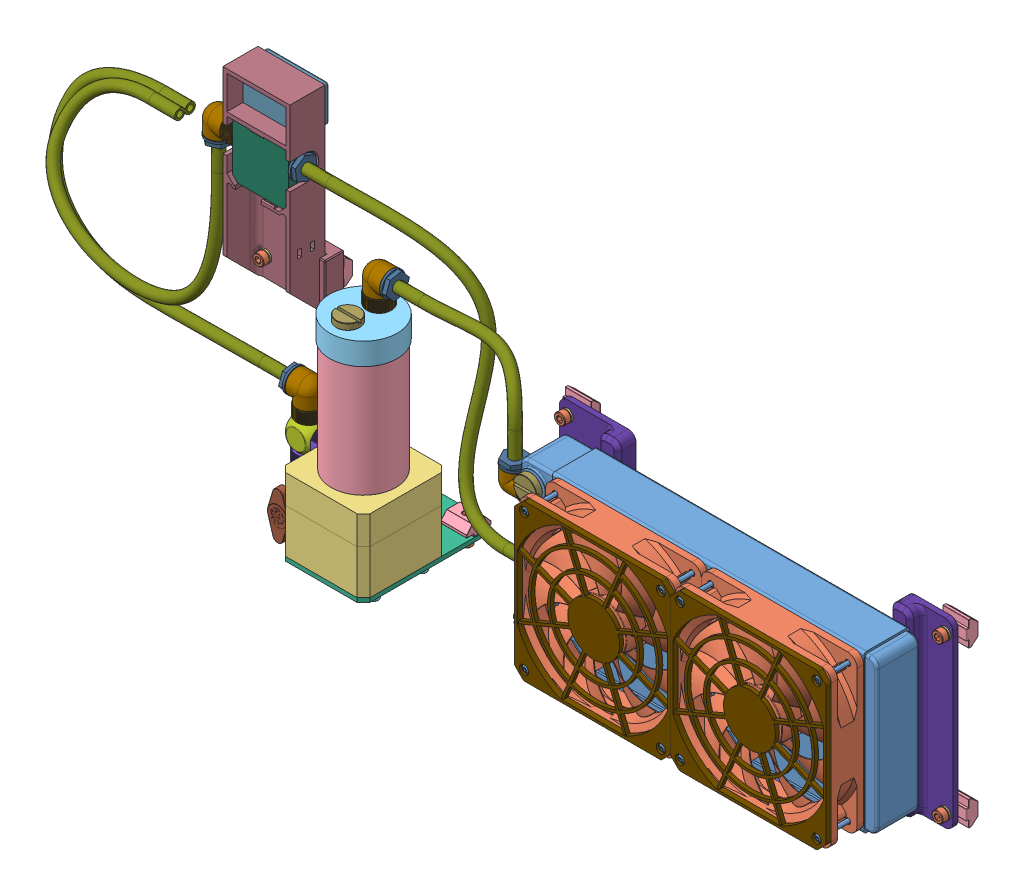
SolidWorks assembly Spindle Cooling Radiator System, configuration Default. Lengths in mm.
Overall size (706.65 292.49 113).
80 component instances, 24 part files, 129 mates.
Components (placement in the parent):
- XSPC EX240 Radiator-1: XSPC EX240 Radiator [Default] at (629 19.5 31.5) x (0 1 0) z (0 0 1) size (121 276 36)
- Noctua_nf-p12 redux-1700-1: Noctua_nf-p12 redux-1700 [Default] at (559.8 79.8 74) x (-1 0 0) z (0 0 -1) size (120 120.2 29.18)
- Noctua_nf-p12 redux-1700-2: Noctua_nf-p12 redux-1700 [Default] at (439.8 79.8 74) x (-1 0 0) z (0 0 -1) size (120 120.2 29.18)
- Cooling Pump-1: Cooling Pump [Default] at (220 0 34.5) x (0 0 1) z (-1 0 0) size (102 211.26 121.52)
  - Freezemod_PU-FS6M-1: Freezemod_PU-FS6M [Default] at origin size (65 159.5 65)
    - Freezemod FS6M_Plus-1: Freezemod FS6M_Plus [Default] at origin size (65 56 65)
    - Freezemod Resevoir-1: Freezemod Resevoir [Default] at (0 99.5 0) x (1 0 0) z (0 1 0) size (52 52 110.5)
      - Innter Tube-1: Innter Tube [Default] at (0 0 99.5) x (1 0 0) z (0 0 -1) size (50 50 100)
      - Top Cap-1: Top Cap [Default] at (0 0 60) x (1 0 0) z (0 0 -1) size (52 52 17)
  - Freezemod PU-FS6M Mounting Bracket-1: Freezemod PU-FS6M Mounting Bracket [Default] at (-18.5 0 0) x (0 0 1) z (0 -1 0) size (65 102 3.17)
  - Bitspower_T_Fitting-1: Bitspower_T_Fitting [Défaut] at (-16.5 43 58.66) x (0 0 1) z (1 0 0) size (25.4 20.32 25.4)
  - EK-AF Extender Rotary M-M G1_4-1: EK-AF Extender Rotary M-M G1_4 [Default] at (-16.5 43 48.5) x (1 0 0) z (0 1 0) size (19.99 25.44 20)
  - EK-AF Angled 90deg G1_4-1: EK-AF Angled 90deg G1_4 [Default] at (-16.5 53.66 58.66) x (-1 0 0) z (0 0 -1) size (19 36.31 19.39)
  - G14x6mm_Barb-1: G14x6mm_Barb [Défaut] at (-16.5 72.46 73.0225) x (0 0 1) z (-0.923728 -0.383049 0) size (25.52 18.33 18.33)
  - EK-AF Extender Rotary M-M G1_4-2: EK-AF Extender Rotary M-M G1_4 [Default] at (-16.5 16.84 58.66) size (19.99 25.44 20)
  - G14_Valve-1: G14_Valve [Predeterminado] at (-16.5 -1.16 58.66) x (0 0 -1) z (0 -1 0) size (23 35.7 37.13)
  - G14_Plug-1: G14_Plug [Default] at (12 165.3 0) x (1 0 0) z (0 -1 0) size (18.01 18.01 9.94)
  - EK-AF Angled 90deg G1_4-3: EK-AF Angled 90deg G1_4 [Default] at (-12 160 0) size (19 36.31 19.39)
  - G14x6mm_Barb-2: G14x6mm_Barb [Défaut] at (-12 178.8 -14.3625) x (0 0 -1) z (-0.216826 -0.97621 0) size (25.52 18.33 18.33)
- G14x6mm_Barb-1: G14x6mm_Barb [Défaut] at (348.2375 55 31.5) x (-1 0 0) z (0 -0.924225 -0.381849) size (25.52 18.33 18.33)
- Flow_Temp_Indicator_ASMB-1: Flow_Temp_Indicator_ASMB [Default] at (140 256.91 10) x (-1 0 0) z (0 0 -1) size (96.24 147.76 37.92)
  - Flow Meter And Temp Gauge-1: Flow Meter And Temp Gauge [Default] at origin size (61.6 147.76 37)
  - Fosa Pointer Display Thermometer-1: Fosa Pointer Display Thermometer [Défaut] at origin size (48 28 20)
  - Fosa G14 Flow Meter-1: Fosa G14 Flow Meter [Default] at (0 -37.73 -4) size (43.25 43.13 20)
  - EK-AF Angled 90deg G1_4-1: EK-AF Angled 90deg G1_4 [Default] at (22.125 -32.1 -15) x (0 0 1) z (0 1 0) size (19 36.31 19.39)
  - G14x6mm_Barb-1: G14x6mm_Barb [Défaut] at (-26.3875 -32.1 -15) x (-1 0 0) z (0 -0.924225 -0.381849) size (25.52 18.33 18.33)
  - G14x6mm_Barb-2: G14x6mm_Barb [Défaut] at (40.925 -46.4625 -15) x (0 -1 0) z (-0.650255 0 0.759716) size (25.52 18.33 18.33)
- EK-AF Angled 90deg G1_4-1: EK-AF Angled 90deg G1_4 [Default] at (352.5 105 31.5) x (0 0 1) z (0 -1 0) size (19 36.31 19.39)
- G14x6mm_Barb-2: G14x6mm_Barb [Défaut] at (333.7 119.3625 31.5) x (0 1 0) z (0 0 1) size (25.52 18.33 18.33)
- Water Cooling Tubes-1: Water Cooling Tubes [Default] at (333.7 119.3625 31.5) x (0 0 -1) z (0 1 0) size (64.89 407.39 178.39)
- G14_Plug-1: G14_Plug [Default] at (365 125 55.3) x (0 1 0) z (0 0 -1) size (18.01 18.01 9.94)
- G14_Plug-2: G14_Plug [Default] at (365 35 55.3) x (-0.158553 0.987351 0) z (0 0 -1) size (18.01 18.01 9.94)
- Radiator Mount-1: Radiator Mount [Outlet Side] at (368 80 0) x (0 1 0) z (0 0 1) size (140 55 14)
- Radiator Mount-2: Radiator Mount [Default] at (624 80 0) x (0 -1 0) z (0 0 1) size (140 39 14)
- Fan_Grill-1: Fan_Grill [Default] at (439.8 79.8 74) size (120 120 4)
- Fan_Grill-2: Fan_Grill [Default] at (559.8 79.8 74) size (120 120 4)
- Trimcraft M3 BSC-1: Trimcraft M3 BSC [3mm x 06mm SST BSC] at (387.5 132.5 9.35) x (-0.923728 -0.383049 0) z (0 0 -1) size (5.7 5.7 7.77)
- Trimcraft M3 BSC-2: Trimcraft M3 BSC [3mm x 06mm SST BSC] at (387.5 27.5 9.35) x (-0.85131 -0.524663 0) z (0 0 -1) size (5.7 5.7 7.77)
- Trimcraft M3 BSC-5: Trimcraft M3 BSC [3mm x 06mm SST BSC] at (612.5 132.5 9.35) x (-0.777574 -0.628792 0) z (0 0 -1) size (5.7 5.7 7.77)
- Trimcraft M3 BSC-7: Trimcraft M3 BSC [3mm x 06mm SST BSC] at (612.5 27.5 9.35) x (-0.715577 -0.698533 0) z (0 0 -1) size (5.7 5.7 7.77)
- Trimcraft M3 BSC-10: Trimcraft M3 BSC [3mm x 30mm SST BSC] at (387.1 27.1 77.65) size (5.7 5.7 31.77)
- Trimcraft M3 BSC-11: Trimcraft M3 BSC [3mm x 30mm SST BSC] at (387.1 132.5 77.65) x (0.987351 0.158553 0) z (0 0 1) size (5.7 5.7 31.77)
- Trimcraft M3 BSC-13: Trimcraft M3 BSC [3mm x 30mm SST BSC] at (492.5 132.5 77.65) x (0.959125 0.282984 0) z (0 0 1) size (5.7 5.7 31.77)
- Trimcraft M3 BSC-15: Trimcraft M3 BSC [3mm x 30mm SST BSC] at (492.5 27.1 77.65) x (0.928571 0.371154 0) z (0 0 1) size (5.7 5.7 31.77)
- Trimcraft M3 BSC-17: Trimcraft M3 BSC [3mm x 30mm SST BSC] at (507.1 27.1 77.65) x (0.906989 0.421154 0) z (0 0 1) size (5.7 5.7 31.77)
- Trimcraft M3 BSC-19: Trimcraft M3 BSC [3mm x 30mm SST BSC] at (507.1 132.5 77.65) x (0.902849 0.429957 0) z (0 0 1) size (5.7 5.7 31.77)
- Trimcraft M3 BSC-21: Trimcraft M3 BSC [3mm x 30mm SST BSC] at (612.5 132.5 77.65) x (0.919615 0.39282 0) z (0 0 1) size (5.7 5.7 31.77)
- Trimcraft M3 BSC-23: Trimcraft M3 BSC [3mm x 30mm SST BSC] at (612.5 27.1 77.65) x (0.952324 0.305088 0) z (0 0 1) size (5.7 5.7 31.77)
- 5mm_SCS_SST-1: 5mm_SCS_SST [5mm SCS SST x 16mm  DIN 912, ISO 4762] at (637.5 140 -10.9) x (-0.923728 -0.383049 0) z (0 0 -1) size (8.5 8.5 21.93)
- 5mm_Washer_SST-1: 5mm_Washer_SST [98689A114] at (637.5 140 5.1) x (-0.923728 -0.383049 0) z (0 0 -1) size (9 9 1.1)
- M5_Tnut_40Series-Profile-1: M5_Tnut_40Series-Profile [Default] at (647.5 140 -2.52) x (0 -1 0) z (-1 0 0) size (19 9 20)
- M5_Tnut_40Series-Profile-2: M5_Tnut_40Series-Profile [Default] at (647.5 20 -2.52) x (0 -1 0) z (-1 0 0) size (19 9 20)
- 5mm_Washer_SST-2: 5mm_Washer_SST [98689A114] at (637.5 20 5.1) x (-0.85131 -0.524663 0) z (0 0 -1) size (9 9 1.1)
- 5mm_SCS_SST-2: 5mm_SCS_SST [5mm SCS SST x 16mm  DIN 912, ISO 4762] at (637.5 20 -10.9) x (-0.85131 -0.524663 0) z (0 0 -1) size (8.5 8.5 21.93)
- M5_Tnut_40Series-Profile-4: M5_Tnut_40Series-Profile [Default] at (356.5 140 -2.52) x (0 -1 0) z (-1 0 0) size (19 9 20)
- 5mm_Washer_SST-4: 5mm_Washer_SST [98689A114] at (346.5 140 5.1) x (-0.777574 -0.628792 0) z (0 0 -1) size (9 9 1.1)
- 5mm_SCS_SST-4: 5mm_SCS_SST [5mm SCS SST x 16mm  DIN 912, ISO 4762] at (346.5 140 -10.9) x (-0.777574 -0.628792 0) z (0 0 -1) size (8.5 8.5 21.93)
- M5_Tnut_40Series-Profile-6: M5_Tnut_40Series-Profile [Default] at (356.5 20 -2.52) x (0 -1 0) z (-1 0 0) size (19 9 20)
- 5mm_Washer_SST-6: 5mm_Washer_SST [98689A114] at (346.5 20 5.1) x (-0.715577 -0.698533 0) z (0 0 -1) size (9 9 1.1)
- 5mm_SCS_SST-6: 5mm_SCS_SST [5mm SCS SST x 16mm  DIN 912, ISO 4762] at (346.5 20 -10.9) x (-0.715577 -0.698533 0) z (0 0 -1) size (8.5 8.5 21.93)
- M5_Tnut_40Series-Profile-8: M5_Tnut_40Series-Profile [Default] at (254.5 2.52 -20) x (0 0 -1) z (-1 0 0) size (19 9 20)
- 5mm_Washer_SST-8: 5mm_Washer_SST [98689A114] at (244.5 -4.275 -20) x (-0.999884 0 0.015211) z (0 1 0) size (9 9 1.1)
- 5mm_SCS_SST-8: 5mm_SCS_SST [5mm SCS SST x 16mm  DIN 912, ISO 4762] at (244.5 11.725 -20) x (-0.999884 0 0.015211) z (0 1 0) size (8.5 8.5 21.93)
- M5_Tnut_40Series-Profile-10: M5_Tnut_40Series-Profile [Default] at (205.5 2.52 -20) x (0 0 -1) z (-1 0 0) size (19 9 20)
- 5mm_Washer_SST-10: 5mm_Washer_SST [98689A114] at (195.5 -4.275 -20) x (-0.973649 0 0.22805) z (0 1 0) size (9 9 1.1)
- 5mm_SCS_SST-10: 5mm_SCS_SST [5mm SCS SST x 16mm  DIN 912, ISO 4762] at (195.5 11.725 -20) x (-0.973649 0 0.22805) z (0 1 0) size (8.5 8.5 21.93)
- 5mm_SCS_SST-12: 5mm_SCS_SST [5mm SCS SST x 25mm  DIN 912, ISO 4762] at (155.8 140 -9.9) x (-0.668041 -0.744124 0) z (0 0 -1) size (8.5 8.5 30.93)
- 5mm_Washer_SST-12: 5mm_Washer_SST [98689A114] at (155.8 140 15.1) x (-0.668041 -0.744124 0) z (0 0 -1) size (9 9 1.1)
- M5_Tnut_40Series-Profile-12: M5_Tnut_40Series-Profile [Default] at (165.8 140 -2.52) x (0 -1 0) z (-1 0 0) size (19 9 20)
- 5mm_SCS_SST-14: 5mm_SCS_SST [5mm SCS SST x 25mm  DIN 912, ISO 4762] at (124.2 140 -9.9) x (-0.567853 -0.82313 0) z (0 0 -1) size (8.5 8.5 30.93)
- 5mm_Washer_SST-14: 5mm_Washer_SST [98689A114] at (124.2 140 15.1) x (-0.567853 -0.82313 0) z (0 0 -1) size (9 9 1.1)
- M5_Tnut_40Series-Profile-14: M5_Tnut_40Series-Profile [Default] at (134.2 140 -2.52) x (0 -1 0) z (-1 0 0) size (19 9 20)
- 4mm_SCS_SST-1: 4mm_SCS_SST [4mm SCS SST x 08mm  DIN 912, ISO 4762] at (246.5 4.225 53) x (1 0 0) z (0 1 0) size (7 7 12.79)
- 4mm_Washer_SST-1: 4mm_Washer_SST [98689A113] at (246.5 -3.775 53) x (1 0 0) z (0 1 0) size (8 8 0.6)
- 4mm_SCS_SST-2: 4mm_SCS_SST [4mm SCS SST x 08mm  DIN 912, ISO 4762] at (246.5 4.225 16) x (0.982082 0 -0.188455) z (0 1 0) size (7 7 12.79)
- 4mm_Washer_SST-2: 4mm_Washer_SST [98689A113] at (246.5 -3.775 16) x (0.982082 0 -0.188455) z (0 1 0) size (8 8 0.6)
- 4mm_SCS_SST-3: 4mm_SCS_SST [4mm SCS SST x 08mm  DIN 912, ISO 4762] at (193.5 4.225 16) x (0.918365 0 -0.395734) z (0 1 0) size (7 7 12.79)
- 4mm_Washer_SST-3: 4mm_Washer_SST [98689A113] at (193.5 -3.775 16) x (0.918365 0 -0.395734) z (0 1 0) size (8 8 0.6)
- 4mm_SCS_SST-4: 4mm_SCS_SST [4mm SCS SST x 08mm  DIN 912, ISO 4762] at (193.5 4.225 53) x (0.8 0 -0.6) z (0 1 0) size (7 7 12.79)
- 4mm_Washer_SST-4: 4mm_Washer_SST [98689A113] at (193.5 -3.775 53) x (0.8 0 -0.6) z (0 1 0) size (8 8 0.6)
Mates (geometry in assembly coordinates):
- Concentric1: concentric: cylinder of XSPC EX240 Radiator-1 through (387.5 132.5 14) axis (0 0 -1) radius 1.3526; cylinder of Radiator Mount-1 through (387.5 132.5 14) axis (0 0 -1) radius 1.75
- Coincident4: coincident: plane of XSPC EX240 Radiator-1 through (629 19.5 14) normal (0 0 -1); plane of Radiator Mount-1 through (368 80 14) normal (0 0 1)
- Parallel2: parallel: plane of Radiator Mount-1 through (395.5 10 4) normal (1 0 0); plane of assembly through (0 0 0) normal (1 0 0)
- Concentric3: concentric: cylinder of XSPC EX240 Radiator-1 through (612.5 132.5 14) axis (0 0 -1) radius 1.3526; cylinder of Radiator Mount-2 through (612.5 132.5 14) axis (0 0 -1) radius 1.75
- Concentric4: concentric: cylinder of XSPC EX240 Radiator-1 through (612.5 27.5 14) axis (0 0 -1) radius 1.3526; cylinder of Radiator Mount-2 through (612.5 27.5 14) axis (0 0 -1) radius 1.75
- Coincident6: coincident: plane of XSPC EX240 Radiator-1 through (629 19.5 14) normal (0 0 -1); plane of Radiator Mount-2 through (624 80 14) normal (0 0 1)
- Concentric5: concentric: cylinder of XSPC EX240 Radiator-1 through (612.5 132.5 49) axis (0 0 1) radius 1.3526; cylinder of Noctua_nf-p12 redux-1700-1 through (612.5 132.5 49) axis (0 0 1) radius 2.2
- Coincident7: coincident: plane of XSPC EX240 Radiator-1 through (629 19.5 49) normal (0 0 1); plane of Noctua_nf-p12 redux-1700-1 through (559.8 79.8 49) normal (0 0 -1)
- Parallel4: parallel: plane of XSPC EX240 Radiator-1 through (629 19.5 31.5) normal (0 1 0); plane of Noctua_nf-p12 redux-1700-1 through (559.8 79.8 74) normal (0 1 0)
- Coincident9: coincident: plane of XSPC EX240 Radiator-1 through (629 19.5 49) normal (0 0 1); plane of Noctua_nf-p12 redux-1700-2 through (439.8 79.8 49) normal (0 0 -1)
- Parallel5: parallel: plane of XSPC EX240 Radiator-1 through (629 19.5 31.5) normal (0 1 0); plane of Noctua_nf-p12 redux-1700-2 through (439.8 79.8 74) normal (0 1 0)
- Concentric8: concentric: cylinder of XSPC EX240 Radiator-1 through (492.5 132.5 49) axis (0 0 1) radius 1.3526; cylinder of Noctua_nf-p12 redux-1700-2 through (492.5 132.5 49) axis (0 0 1) radius 2.2
- Concentric9: concentric: cylinder of XSPC EX240 Radiator-1 through (357 55 31.5) axis (-1 0 0) radius 6.5785; cylinder of G14x6mm_Barb-1 through (357.7625 55 31.5) axis (-1 0 0) radius 6.5786
- Coincident12: coincident: plane of XSPC EX240 Radiator-1 through (353 55 31.5) normal (-1 0 0); plane of G14x6mm_Barb-1 through (353 55 31.5) normal (1 0 0)
- Concentric10: concentric: cylinder of XSPC EX240 Radiator-1 through (357 105 31.5) axis (-1 0 0) radius 6.5785; cylinder of EK-AF Angled 90deg G1_4-1 through (343.45 105 31.5) axis (1 0 0) radius 5.25
- Coincident13: coincident: plane of XSPC EX240 Radiator-1 through (353 105 31.5) normal (-1 0 0); plane of EK-AF Angled 90deg G1_4-1 through (353 105 23.9) normal (1 0 0)
- Concentric11: concentric: cylinder of EK-AF Angled 90deg G1_4-1 through (333.7 114.6 31.5) axis (0 -1 0) radius 9; cylinder of G14x6mm_Barb-2 through (333.7 109.8375 31.5) axis (0 1 0) radius 6.5786
- Coincident15: coincident: plane of EK-AF Angled 90deg G1_4-1 through (333.7 114.6 31.5) normal (0 1 0); plane of G14x6mm_Barb-2 through (333.7 114.6 31.5) normal (0 -1 0)
- Coincident16: coincident: plane of Radiator Mount-1 through (368 80 0) normal (0 0 -1); plane of assembly through (0 0 0) normal (0 0 1)
- Coincident18: coincident: point of Radiator Mount-1; line of assembly
- Coincident20: coincident: plane of Cooling Pump-1/Freezemod PU-FS6M Mounting Bracket-1 through (220 0 16) normal (0 1 0); plane of assembly through (0 0 0) normal (0 1 0)
- Coincident21: coincident: line of Cooling Pump-1/Freezemod PU-FS6M Mounting Bracket-1 through (252.5 0 -20) axis (-1 0 0); line of assembly
- Coincident22: coincident: plane of Flow_Temp_Indicator_ASMB-1/Flow Meter And Temp Gauge-1 through (140 256.91 0) normal (0 0 -1); plane of assembly through (0 0 0) normal (0 0 1)
- Coincident26: coincident: line of ? through (155.8 140 0) axis (-1 0 0)
- Distance4: distance = 500 mm: plane of XSPC EX240 Radiator-1 through (500 19.5 31.5) normal (-1 0 0); plane of assembly through (0 0 0) normal (1 0 0)
- Distance5: distance = 220 mm: plane of Cooling Pump-1/Freezemod_PU-FS6M-1/Freezemod FS6M_Plus-1 through (220 0 34.5) normal (-1 0 0); plane of assembly through (0 0 0) normal (1 0 0)
- Distance6: distance = 140 mm: plane of ? through (140 256.91 10) normal (-1 0 0); plane of assembly through (0 0 0) normal (1 0 0)
- Coincident33: coincident: plane of Noctua_nf-p12 redux-1700-2 through (439.8 79.8 74) normal (0 0 1); plane of Fan_Grill-1 through (439.8 79.8 74) normal (0 0 -1)
- Coincident34: coincident: plane of Noctua_nf-p12 redux-1700-1 through (559.8 79.8 74) normal (0 0 1); plane of Fan_Grill-2 through (559.8 79.8 74) normal (0 0 -1)
- Concentric12: concentric: cylinder of Noctua_nf-p12 redux-1700-2 through (387.1 132.5 49) axis (0 0 1) radius 2.2; cylinder of Fan_Grill-1 through (387.1 132.5 78) axis (0 0 -1) radius 2.15
- Concentric15: concentric: cylinder of Noctua_nf-p12 redux-1700-2 through (492.5 27.1 49) axis (0 0 1) radius 2.2; cylinder of Fan_Grill-1 through (492.5 27.1 78) axis (0 0 -1) radius 2.15
- Concentric16: concentric: cylinder of Noctua_nf-p12 redux-1700-1 through (507.1 132.5 49) axis (0 0 1) radius 2.2; cylinder of Fan_Grill-2 through (507.1 132.5 78) axis (0 0 -1) radius 2.15
- Concentric17: concentric: cylinder of Noctua_nf-p12 redux-1700-1 through (612.5 27.1 49) axis (0 0 1) radius 2.2; cylinder of Fan_Grill-2 through (612.5 27.1 78) axis (0 0 -1) radius 2.15
- InPlace1: in place: plane of G14x6mm_Barb-2 through (333.7 119.3625 31.5) normal (0 1 0); plane of ? through (0 119.3625 0) normal (0 1 0); moOrthogonalPlaneRef_w of G14x6mm_Barb-2 through (333.7 119.3625 31.5) normal (0 1 0); plane of ? through (0 119.3625 0) normal (0 0 -1); plane of G14x6mm_Barb-2 through (333.7 119.3625 31.5) normal (0 1 0); plane of ? through (0 119.3625 0) normal (1 0 0); plane of G14x6mm_Barb-2 through (333.7 119.3625 31.5) normal (0 1 0); unknown of Water Cooling Tubes-1
- Coincident35: coincident: plane of G14x6mm_Barb-2; plane of Water Cooling Tubes-1
- Coincident36: coincident: moOrthogonalPlaneRef_w of G14x6mm_Barb-2 through (333.7 119.3625 31.5) normal (-1 0 0); plane of Water Cooling Tubes-1 through (333.7 119.3625 31.5) normal (-1 0 0)
- Coincident37: coincident: moOrthogonalPlaneRef_w of G14x6mm_Barb-2 through (333.7 119.3625 31.5) normal (0 0 1); plane of Water Cooling Tubes-1 through (333.7 119.3625 31.5) normal (0 0 -1)
- Concentric18: concentric: cylinder of XSPC EX240 Radiator-1 through (365 125 45.5) axis (0 0 1) radius 6.5785; cylinder of G14_Plug-1 through (365 125 45.5) axis (0 0 1) radius 5.9
- Tangent1: tangent: plane of XSPC EX240 Radiator-1 through (629 19.5 49.5) normal (0 0 1); face of G14_Plug-1
- Concentric19: concentric: cylinder of XSPC EX240 Radiator-1 through (365 35 45.5) axis (0 0 1) radius 6.5785; cylinder of G14_Plug-2 through (365 35 45.5) axis (0 0 1) radius 5.9
- Tangent2: tangent: plane of XSPC EX240 Radiator-1 through (629 19.5 49.5) normal (0 0 1); face of G14_Plug-2
- Concentric20: concentric: cylinder of XSPC EX240 Radiator-1 through (387.5 132.5 14) axis (0 0 -1) radius 1.3526; cylinder of Trimcraft M3 BSC-1 through (387.5 132.5 17) axis (0 0 1) radius 1.5
- Coincident36: coincident: plane of Radiator Mount-1 through (368 80 11) normal (0 0 -1); plane of Trimcraft M3 BSC-1 through (388.5917 129.8674 11) normal (0 0 1)
- Coincident37: coincident: plane of Radiator Mount-1 through (368 80 11) normal (0 0 -1); plane of Trimcraft M3 BSC-2 through (388.9953 25.0738 11) normal (0 0 1)
- Concentric21: concentric: cylinder of XSPC EX240 Radiator-1 through (387.5 27.5 14) axis (0 0 -1) radius 1.3526; cylinder of Trimcraft M3 BSC-2 through (387.5 27.5 17) axis (0 0 1) radius 1.5
- Concentric22: concentric: cylinder of XSPC EX240 Radiator-1 through (612.5 132.5 14) axis (0 0 -1) radius 1.3526; cylinder of Trimcraft M3 BSC-5 through (612.5 132.5 17) axis (0 0 1) radius 1.5
- Concentric23: concentric: cylinder of XSPC EX240 Radiator-1 through (612.5 27.5 14) axis (0 0 -1) radius 1.3526; cylinder of Trimcraft M3 BSC-7 through (612.5 27.5 17) axis (0 0 1) radius 1.5
- Coincident39: coincident: plane of Radiator Mount-2 through (624 80 11) normal (0 0 -1); plane of Trimcraft M3 BSC-5 through (614.2921 130.2839 11) normal (0 0 1)
- Coincident40: coincident: plane of Radiator Mount-2 through (624 80 11) normal (0 0 -1); plane of Trimcraft M3 BSC-7 through (614.4908 25.4606 11) normal (0 0 1)
- Concentric24: concentric: cylinder of Fan_Grill-1 through (387.1 27.1 78) axis (0 0 -1) radius 2.15; cylinder of Trimcraft M3 BSC-10 through (387.1 27.1 46) axis (0 0 -1) radius 1.5
- Coincident41: coincident: plane of Fan_Grill-1 through (387.1 27.1 76) normal (0 0 1); plane of Trimcraft M3 BSC-10 through (387.1 24.25 76) normal (0 0 -1)
- Concentric25: concentric: cylinder of Fan_Grill-1 through (387.1 132.5 78) axis (0 0 -1) radius 2.15; cylinder of Trimcraft M3 BSC-11 through (387.1 132.5 46) axis (0 0 -1) radius 1.5
- Coincident42: coincident: plane of Fan_Grill-1 through (387.1 132.5 76) normal (0 0 1); plane of Trimcraft M3 BSC-11 through (387.5519 129.6861 76) normal (0 0 -1)
- Concentric26: concentric: cylinder of Fan_Grill-1 through (492.5 132.5 78) axis (0 0 -1) radius 2.15; cylinder of Trimcraft M3 BSC-13 through (492.5 132.5 46) axis (0 0 -1) radius 1.5
- Coincident43: coincident: plane of Fan_Grill-1 through (492.5 132.5 76) normal (0 0 1); plane of Trimcraft M3 BSC-13 through (493.3065 129.7665 76) normal (0 0 -1)
- Concentric27: concentric: cylinder of Fan_Grill-1 through (492.5 27.1 78) axis (0 0 -1) radius 2.15; cylinder of Trimcraft M3 BSC-15 through (492.5 27.1 46) axis (0 0 -1) radius 1.5
- Coincident44: coincident: plane of Fan_Grill-1 through (492.5 27.1 76) normal (0 0 1); plane of Trimcraft M3 BSC-15 through (493.5578 24.4536 76) normal (0 0 -1)
- Concentric28: concentric: cylinder of Fan_Grill-2 through (507.1 27.1 78) axis (0 0 -1) radius 2.15; cylinder of Trimcraft M3 BSC-17 through (507.1 27.1 46) axis (0 0 -1) radius 1.5
- Coincident45: coincident: plane of Fan_Grill-2 through (507.1 27.1 76) normal (0 0 1); plane of Trimcraft M3 BSC-17 through (508.3003 24.5151 76) normal (0 0 -1)
- Concentric29: concentric: cylinder of Fan_Grill-2 through (507.1 132.5 78) axis (0 0 -1) radius 2.15; cylinder of Trimcraft M3 BSC-19 through (507.1 132.5 46) axis (0 0 -1) radius 1.5
- Coincident46: coincident: plane of Fan_Grill-2 through (507.1 132.5 76) normal (0 0 1); plane of Trimcraft M3 BSC-19 through (508.3254 129.9269 76) normal (0 0 -1)
- Concentric30: concentric: cylinder of Fan_Grill-2 through (612.5 132.5 78) axis (0 0 -1) radius 2.15; cylinder of Trimcraft M3 BSC-21 through (612.5 132.5 46) axis (0 0 -1) radius 1.5
- Coincident47: coincident: plane of Fan_Grill-2 through (612.5 132.5 76) normal (0 0 1); plane of Trimcraft M3 BSC-21 through (613.6195 129.8791 76) normal (0 0 -1)
- Concentric31: concentric: cylinder of Fan_Grill-2 through (612.5 27.1 78) axis (0 0 -1) radius 2.15; cylinder of Trimcraft M3 BSC-23 through (612.5 27.1 46) axis (0 0 -1) radius 1.5
- Coincident48: coincident: plane of Fan_Grill-2 through (612.5 27.1 76) normal (0 0 1); plane of Trimcraft M3 BSC-23 through (613.3695 24.3859 76) normal (0 0 -1)
- Concentric32: concentric: cylinder of 5mm_SCS_SST-1 through (637.5 140 5.1) axis (0 0 -1) radius 2.5; cylinder of 5mm_Washer_SST-1 through (637.5 140 4) axis (0 0 1) radius 2.65
- Coincident49: coincident: plane of 5mm_SCS_SST-1 through (637.5 140 5.1) normal (0 0 -1); plane of 5mm_Washer_SST-1 through (637.5 140 5.1) normal (0 0 1)
- Concentric33: concentric: cylinder of Radiator Mount-2 through (637.5 140 4) axis (0 0 -1) radius 2.65; cylinder of 5mm_SCS_SST-1 through (637.5 140 5.1) axis (0 0 -1) radius 2.5
- Coincident50: coincident: plane of Radiator Mount-2 through (624 80 4) normal (0 0 1); plane of 5mm_Washer_SST-1 through (637.5 140 4) normal (0 0 -1)
- Concentric34: concentric: cylinder of 5mm_SCS_SST-1 through (637.5 140 5.1) axis (0 0 -1) radius 2.5; cylinder of M5_Tnut_40Series-Profile-1 through (637.5 140 -2.52) axis (0 0 1) radius 2.1
- Distance7: distance = 4.32 mm: plane of M5_Tnut_40Series-Profile-1 through (627.5 144 -4.32) normal (0 0 1); plane of Radiator Mount-2 through (624 80 0) normal (0 0 -1)
- Concentric35: concentric: cylinder of 5mm_Washer_SST-2 through (637.5 20 4) axis (0 0 1) radius 2.65; cylinder of 5mm_SCS_SST-2 through (637.5 20 5.1) axis (0 0 -1) radius 2.5
- Coincident53: coincident: plane of 5mm_Washer_SST-2 through (637.5 20 5.1) normal (0 0 1); plane of 5mm_SCS_SST-2 through (637.5 20 5.1) normal (0 0 -1)
- Concentric36: concentric: cylinder of M5_Tnut_40Series-Profile-2 through (637.5 20 -2.52) axis (0 0 1) radius 2.1; cylinder of 5mm_SCS_SST-2 through (637.5 20 5.1) axis (0 0 -1) radius 2.5
- Concentric37: concentric: cylinder of Radiator Mount-2 through (637.5 20 4) axis (0 0 -1) radius 2.65; cylinder of 5mm_SCS_SST-2 through (637.5 20 5.1) axis (0 0 -1) radius 2.5
- Coincident54: coincident: plane of Radiator Mount-2 through (624 80 4) normal (0 0 1); plane of 5mm_Washer_SST-2 through (637.5 20 4) normal (0 0 -1)
- Distance8: distance = 4.32 mm: plane of M5_Tnut_40Series-Profile-2 through (627.5 24 -4.32) normal (0 0 1); plane of Radiator Mount-2 through (624 80 0) normal (0 0 -1)
- Concentric40: concentric: cylinder of 5mm_Washer_SST-4 through (346.5 140 4) axis (0 0 1) radius 2.65; cylinder of 5mm_SCS_SST-4 through (346.5 140 5.1) axis (0 0 -1) radius 2.5
- Coincident56: coincident: plane of 5mm_Washer_SST-4 through (346.5 140 5.1) normal (0 0 1); plane of 5mm_SCS_SST-4 through (346.5 140 5.1) normal (0 0 -1)
- Concentric41: concentric: cylinder of M5_Tnut_40Series-Profile-4 through (346.5 140 -2.52) axis (0 0 1) radius 2.1; cylinder of 5mm_SCS_SST-4 through (346.5 140 5.1) axis (0 0 -1) radius 2.5
- Concentric42: concentric: cylinder of Radiator Mount-1 through (346.5 140 4) axis (0 0 -1) radius 2.65; cylinder of 5mm_SCS_SST-4 through (346.5 140 5.1) axis (0 0 -1) radius 2.5
- Coincident57: coincident: plane of Radiator Mount-1 through (368 80 4) normal (0 0 1); plane of 5mm_Washer_SST-4 through (346.5 140 4) normal (0 0 -1)
- Distance9: distance = 4.32 mm: plane of M5_Tnut_40Series-Profile-4 through (336.5 144 -4.32) normal (0 0 1); plane of Radiator Mount-1 through (368 80 0) normal (0 0 -1)
- Concentric45: concentric: cylinder of 5mm_Washer_SST-6 through (346.5 20 4) axis (0 0 1) radius 2.65; cylinder of 5mm_SCS_SST-6 through (346.5 20 5.1) axis (0 0 -1) radius 2.5
- Coincident59: coincident: plane of 5mm_Washer_SST-6 through (346.5 20 5.1) normal (0 0 1); plane of 5mm_SCS_SST-6 through (346.5 20 5.1) normal (0 0 -1)
- Concentric46: concentric: cylinder of M5_Tnut_40Series-Profile-6 through (346.5 20 -2.52) axis (0 0 1) radius 2.1; cylinder of 5mm_SCS_SST-6 through (346.5 20 5.1) axis (0 0 -1) radius 2.5
- Concentric47: concentric: cylinder of Radiator Mount-1 through (346.5 20 4) axis (0 0 -1) radius 2.65; cylinder of 5mm_SCS_SST-6 through (346.5 20 5.1) axis (0 0 -1) radius 2.5
- Coincident60: coincident: plane of Radiator Mount-1 through (368 80 4) normal (0 0 1); plane of 5mm_Washer_SST-6 through (346.5 20 4) normal (0 0 -1)
- Distance10: distance = 4.32 mm: plane of M5_Tnut_40Series-Profile-6 through (336.5 24 -4.32) normal (0 0 1); plane of Radiator Mount-1 through (368 80 0) normal (0 0 -1)
- Concentric50: concentric: cylinder of 5mm_Washer_SST-8 through (244.5 -3.175 -20) axis (0 -1 0) radius 2.65; cylinder of 5mm_SCS_SST-8 through (244.5 -4.275 -20) axis (0 1 0) radius 2.5
- Coincident62: coincident: plane of 5mm_Washer_SST-8 through (244.5 -4.275 -20) normal (0 -1 0); plane of 5mm_SCS_SST-8 through (244.5 -4.275 -20) normal (0 1 0)
- Concentric51: concentric: cylinder of M5_Tnut_40Series-Profile-8 through (244.5 2.52 -20) axis (0 -1 0) radius 2.1; cylinder of 5mm_SCS_SST-8 through (244.5 -4.275 -20) axis (0 1 0) radius 2.5
- Concentric52: concentric: cylinder of Cooling Pump-1/Freezemod PU-FS6M Mounting Bracket-1 through (244.5 -3.175 -20) axis (0 1 0) radius 2.5; cylinder of 5mm_SCS_SST-8 through (244.5 -4.275 -20) axis (0 1 0) radius 2.5
- Coincident63: coincident: plane of Cooling Pump-1/Freezemod PU-FS6M Mounting Bracket-1 through (220 -3.175 16) normal (0 -1 0); plane of 5mm_Washer_SST-8 through (244.5 -3.175 -20) normal (0 1 0)
- Distance11: distance = 4.32 mm: plane of M5_Tnut_40Series-Profile-8 through (234.5 4.32 -16) normal (0 -1 0); plane of Cooling Pump-1/Freezemod PU-FS6M Mounting Bracket-1 through (220 0 16) normal (0 1 0)
- Concentric55: concentric: cylinder of 5mm_Washer_SST-10 through (195.5 -3.175 -20) axis (0 -1 0) radius 2.65; cylinder of 5mm_SCS_SST-10 through (195.5 -4.275 -20) axis (0 1 0) radius 2.5
- Coincident65: coincident: plane of 5mm_Washer_SST-10 through (195.5 -4.275 -20) normal (0 -1 0); plane of 5mm_SCS_SST-10 through (195.5 -4.275 -20) normal (0 1 0)
- Concentric56: concentric: cylinder of M5_Tnut_40Series-Profile-10 through (195.5 2.52 -20) axis (0 -1 0) radius 2.1; cylinder of 5mm_SCS_SST-10 through (195.5 -4.275 -20) axis (0 1 0) radius 2.5
- Concentric57: concentric: cylinder of Cooling Pump-1/Freezemod PU-FS6M Mounting Bracket-1 through (195.5 -3.175 -20) axis (0 1 0) radius 2.5; cylinder of 5mm_SCS_SST-10 through (195.5 -4.275 -20) axis (0 1 0) radius 2.5
- Coincident66: coincident: plane of Cooling Pump-1/Freezemod PU-FS6M Mounting Bracket-1 through (220 -3.175 16) normal (0 -1 0); plane of 5mm_Washer_SST-10 through (195.5 -3.175 -20) normal (0 1 0)
- Distance12: distance = 4.32 mm: plane of M5_Tnut_40Series-Profile-10 through (185.5 4.32 -16) normal (0 -1 0); plane of Cooling Pump-1/Freezemod PU-FS6M Mounting Bracket-1 through (220 0 16) normal (0 1 0)
- Concentric60: concentric: cylinder of 5mm_SCS_SST-12 through (155.8 140 15.1) axis (0 0 -1) radius 2.5; cylinder of 5mm_Washer_SST-12 through (155.8 140 14) axis (0 0 1) radius 2.65
- Coincident73: coincident: plane of 5mm_SCS_SST-12 through (155.8 140 15.1) normal (0 0 -1); plane of 5mm_Washer_SST-12 through (155.8 140 15.1) normal (0 0 1)
- Concentric61: concentric: cylinder of 5mm_SCS_SST-12 through (155.8 140 15.1) axis (0 0 -1) radius 2.5; cylinder of M5_Tnut_40Series-Profile-12 through (155.8 140 -2.52) axis (0 0 1) radius 2.1
- Concentric62: concentric: cylinder of Flow_Temp_Indicator_ASMB-1/Flow Meter And Temp Gauge-1 through (155.8 140 14) axis (0 0 -1) radius 2.65; cylinder of 5mm_SCS_SST-12 through (155.8 140 15.1) axis (0 0 -1) radius 2.5
- Coincident74: coincident: plane of Flow_Temp_Indicator_ASMB-1/Flow Meter And Temp Gauge-1 through (140 256.91 14) normal (0 0 1); plane of 5mm_Washer_SST-12 through (155.8 140 14) normal (0 0 -1)
- Distance13: distance = 4.32 mm: plane of M5_Tnut_40Series-Profile-12 through (145.8 144 -4.32) normal (0 0 1); plane of Flow_Temp_Indicator_ASMB-1/Flow Meter And Temp Gauge-1 through (140 256.91 0) normal (0 0 -1)
- Concentric65: concentric: cylinder of 5mm_SCS_SST-14 through (124.2 140 15.1) axis (0 0 -1) radius 2.5; cylinder of 5mm_Washer_SST-14 through (124.2 140 14) axis (0 0 1) radius 2.65
- Coincident76: coincident: plane of 5mm_SCS_SST-14 through (124.2 140 15.1) normal (0 0 -1); plane of 5mm_Washer_SST-14 through (124.2 140 15.1) normal (0 0 1)
- Concentric66: concentric: cylinder of 5mm_SCS_SST-14 through (124.2 140 15.1) axis (0 0 -1) radius 2.5; cylinder of M5_Tnut_40Series-Profile-14 through (124.2 140 -2.52) axis (0 0 1) radius 2.1
- Concentric67: concentric: cylinder of Flow_Temp_Indicator_ASMB-1/Flow Meter And Temp Gauge-1 through (124.2 140 14) axis (0 0 -1) radius 2.65; cylinder of 5mm_SCS_SST-14 through (124.2 140 15.1) axis (0 0 -1) radius 2.5
- Coincident77: coincident: plane of Flow_Temp_Indicator_ASMB-1/Flow Meter And Temp Gauge-1 through (140 256.91 14) normal (0 0 1); plane of 5mm_Washer_SST-14 through (124.2 140 14) normal (0 0 -1)
- Distance14: distance = 4.32 mm: plane of M5_Tnut_40Series-Profile-14 through (114.2 144 -4.32) normal (0 0 1); plane of Flow_Temp_Indicator_ASMB-1/Flow Meter And Temp Gauge-1 through (140 256.91 0) normal (0 0 -1)
- Concentric70: concentric: cylinder of 4mm_SCS_SST-1 through (246.5 -3.775 53) axis (0 1 0) radius 2; cylinder of 4mm_Washer_SST-1 through (246.5 -3.175 53) axis (0 -1 0) radius 2.15
- Coincident81: coincident: plane of 4mm_SCS_SST-1 through (246.5 -3.775 53) normal (0 1 0); plane of 4mm_Washer_SST-1 through (246.5 -3.775 53) normal (0 -1 0)
- Coincident82: coincident: plane of Cooling Pump-1/Freezemod PU-FS6M Mounting Bracket-1 through (220 -3.175 16) normal (0 -1 0); plane of 4mm_Washer_SST-1 through (246.5 -3.175 53) normal (0 1 0)
- Concentric71: concentric: cylinder of Cooling Pump-1/Freezemod PU-FS6M Mounting Bracket-1 through (246.5 -3.175 53) axis (0 1 0) radius 2; cylinder of 4mm_SCS_SST-1 through (246.5 -3.775 53) axis (0 1 0) radius 2
- Concentric72: concentric: cylinder of 4mm_SCS_SST-2 through (246.5 -3.775 16) axis (0 1 0) radius 2; cylinder of 4mm_Washer_SST-2 through (246.5 -3.175 16) axis (0 -1 0) radius 2.15
- Coincident83: coincident: plane of 4mm_SCS_SST-2 through (246.5 -3.775 16) normal (0 1 0); plane of 4mm_Washer_SST-2 through (246.5 -3.775 16) normal (0 -1 0)
- Coincident84: coincident: plane of Cooling Pump-1/Freezemod PU-FS6M Mounting Bracket-1 through (220 -3.175 16) normal (0 -1 0); plane of 4mm_Washer_SST-2 through (246.5 -3.175 16) normal (0 1 0)
- Concentric73: concentric: cylinder of Cooling Pump-1/Freezemod PU-FS6M Mounting Bracket-1 through (246.5 -3.175 16) axis (0 1 0) radius 2; cylinder of 4mm_SCS_SST-2 through (246.5 -3.775 16) axis (0 1 0) radius 2
- Concentric74: concentric: cylinder of 4mm_SCS_SST-3 through (193.5 -3.775 16) axis (0 1 0) radius 2; cylinder of 4mm_Washer_SST-3 through (193.5 -3.175 16) axis (0 -1 0) radius 2.15
- Coincident85: coincident: plane of 4mm_SCS_SST-3 through (193.5 -3.775 16) normal (0 1 0); plane of 4mm_Washer_SST-3 through (193.5 -3.775 16) normal (0 -1 0)
- Coincident86: coincident: plane of Cooling Pump-1/Freezemod PU-FS6M Mounting Bracket-1 through (220 -3.175 16) normal (0 -1 0); plane of 4mm_Washer_SST-3 through (193.5 -3.175 16) normal (0 1 0)
- Concentric75: concentric: cylinder of Cooling Pump-1/Freezemod PU-FS6M Mounting Bracket-1 through (193.5 -3.175 16) axis (0 1 0) radius 2; cylinder of 4mm_SCS_SST-3 through (193.5 -3.775 16) axis (0 1 0) radius 2
- Concentric76: concentric: cylinder of 4mm_SCS_SST-4 through (193.5 -3.775 53) axis (0 1 0) radius 2; cylinder of 4mm_Washer_SST-4 through (193.5 -3.175 53) axis (0 -1 0) radius 2.15
- Coincident87: coincident: plane of 4mm_SCS_SST-4 through (193.5 -3.775 53) normal (0 1 0); plane of 4mm_Washer_SST-4 through (193.5 -3.775 53) normal (0 -1 0)
- Coincident88: coincident: plane of Cooling Pump-1/Freezemod PU-FS6M Mounting Bracket-1 through (220 -3.175 16) normal (0 -1 0); plane of 4mm_Washer_SST-4 through (193.5 -3.175 53) normal (0 1 0)
- Concentric77: concentric: cylinder of Cooling Pump-1/Freezemod PU-FS6M Mounting Bracket-1 through (193.5 -3.175 53) axis (0 1 0) radius 2; cylinder of 4mm_SCS_SST-4 through (193.5 -3.775 53) axis (0 1 0) radius 2
